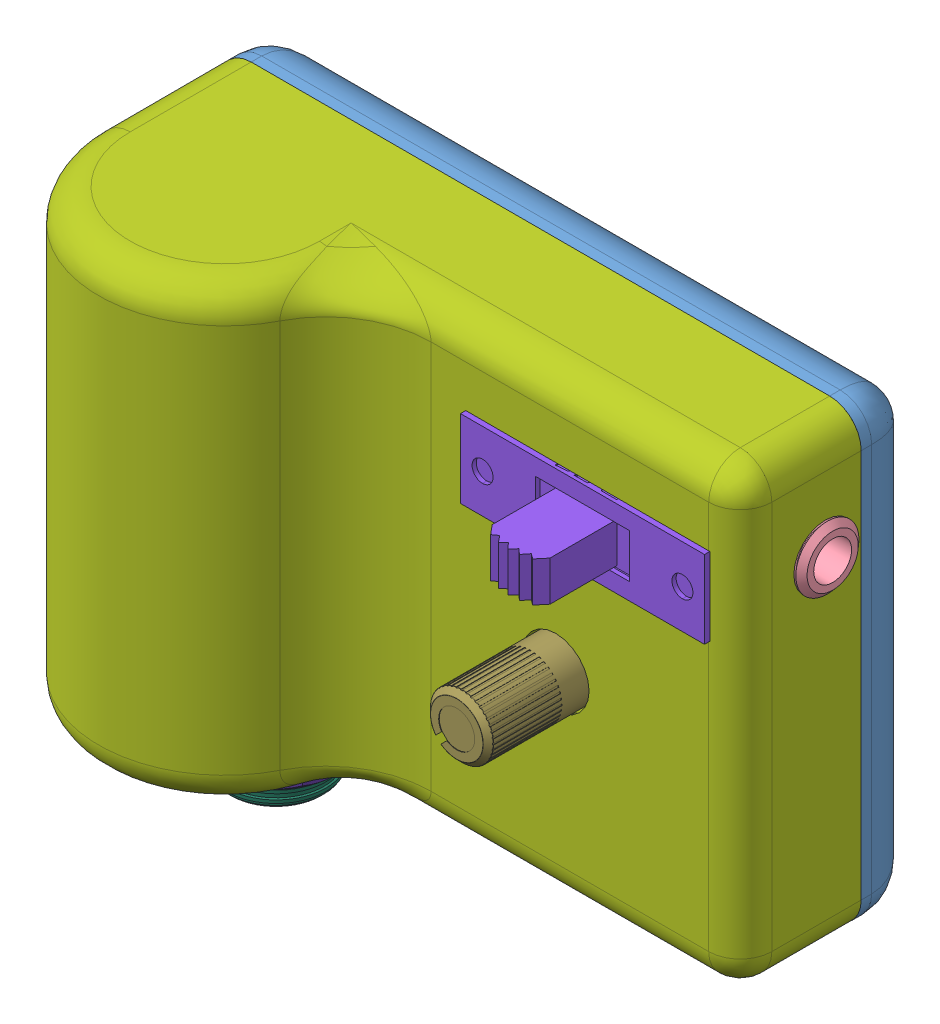
SolidWorks assembly Assem1, configuration Default. Lengths in mm.
Overall size (61.7 49.06 31.9).
226 component instances, 80 part files, 10 mates.
Components (placement in the parent):
- base-1: base [Default] at (33.6508 33.2702 54.2256) size (61 43 11.4)
- Guitar_Headphone_Amp.step-1: Guitar_Headphone_Amp.step [Default] at (133.3435 -10.8718 60.6371) x (0 1 0) z (0 0 1) size (46.1 58.51 24.5)
  - Board.step-1: Board.step [Default] at origin size (37.48 55.26 0.45)
    - Open CASCADE STEP translator 6.8 1.1.1.step-1: Open CASCADE STEP translator 6.8 1.1.1.step [Default] at (0 0 -0.4115) size (37.48 55.26 0.45)
  - U1.step-1: U1.step [Default] at origin size (4 8.8 1.65)
    - 7526814176.step-1: 7526814176.step [Default] at (43.244 100.584 0.1) size (4 8.8 1.65)
      - Extruded.step-1: Extruded.step [Default] at origin size (4 8.8 1.65)
  - R19.step-1: R19.step [Default] at origin size (0.95 1.75 0.55)
    - 7442988304.step-1: 7442988304.step [Default] at (53.086 89.244 0) size (0.95 0.3 0.55)
      - Extruded-0.step-1: Extruded-0.step [Default] at origin size (0.95 0.3 0.55)
    - 7442988304.step-2: 7442988304.step [Default] at (53.086 87.794 0) size (0.95 0.3 0.55)
      - Extruded-0.step-1: Extruded-0.step [Default] at origin size (0.95 0.3 0.55)
    - 7442988144.step-1: 7442988144.step [Default] at (53.086 88.519 0) size (0.95 1.15 0.55)
      - Extruded-1.step-1: Extruded-1.step [Default] at origin size (0.95 1.15 0.55)
  - R18.step-1: R18.step [Default] at origin size (0.95 1.75 0.55)
    - 7442988304.step-1: 7442988304.step [Default] at (57.912 89.244 0) size (0.95 0.3 0.55)
      - Extruded-0.step-1: Extruded-0.step [Default] at origin size (0.95 0.3 0.55)
    - 7442988304.step-2: 7442988304.step [Default] at (57.912 87.794 0) size (0.95 0.3 0.55)
      - Extruded-0.step-1: Extruded-0.step [Default] at origin size (0.95 0.3 0.55)
    - 7442988144.step-1: 7442988144.step [Default] at (57.912 88.519 0) size (0.95 1.15 0.55)
      - Extruded-1.step-1: Extruded-1.step [Default] at origin size (0.95 1.15 0.55)
  - R17.step-1: R17.step [Default] at origin size (1.45 2.2 0.7)
    - 7527189808.step-1: 7527189808.step [Default] at (27.005 91.313 0) size (1.45 1.4 0.7)
      - Extruded-2.step-1: Extruded-2.step [Default] at origin size (1.45 1.4 0.7)
    - 6967077248.step-1: 6967077248.step [Default] at (27.005 90.413 0) size (1.45 0.4 0.7)
      - Extruded-3.step-1: Extruded-3.step [Default] at origin size (1.45 0.4 0.7)
    - 6967077248.step-2: 6967077248.step [Default] at (27.005 92.213 0) size (1.45 0.4 0.7)
      - Extruded-3.step-1: Extruded-3.step [Default] at origin size (1.45 0.4 0.7)
  - R16.step-1: R16.step [Default] at origin size (1.45 2.2 0.6)
    - 7687205168.step-1: 7687205168.step [Default] at (31.7541 82.031 0) size (1.45 0.4 0.6)
      - Extruded-4.step-1: Extruded-4.step [Default] at origin size (1.45 0.4 0.6)
    - 7687205168.step-2: 7687205168.step [Default] at (31.7541 83.831 0) size (1.45 0.4 0.6)
      - Extruded-4.step-1: Extruded-4.step [Default] at origin size (1.45 0.4 0.6)
    - 7687201248.step-1: 7687201248.step [Default] at (31.7541 82.931 0) size (1.45 1.4 0.6)
      - Extruded-5.step-1: Extruded-5.step [Default] at origin size (1.45 1.4 0.6)
  - R15.step-1: R15.step [Default] at origin size (1.45 2.2 0.7)
    - 6967077248.step-1: 6967077248.step [Default] at (27.155 83.301 0) size (1.45 0.4 0.7)
      - Extruded-3.step-1: Extruded-3.step [Default] at origin size (1.45 0.4 0.7)
    - 6967077248.step-2: 6967077248.step [Default] at (27.155 85.101 0) size (1.45 0.4 0.7)
      - Extruded-3.step-1: Extruded-3.step [Default] at origin size (1.45 0.4 0.7)
    - 7527189808.step-1: 7527189808.step [Default] at (27.155 84.201 0) size (1.45 1.4 0.7)
      - Extruded-2.step-1: Extruded-2.step [Default] at origin size (1.45 1.4 0.7)
  - R14.step-1: R14.step [Default] at origin size (1.45 2.2 0.7)
    - 6967077248.step-1: 6967077248.step [Default] at (32.0541 86.095 0) size (1.45 0.4 0.7)
      - Extruded-3.step-1: Extruded-3.step [Default] at origin size (1.45 0.4 0.7)
    - 6967077248.step-2: 6967077248.step [Default] at (32.0541 87.895 0) size (1.45 0.4 0.7)
      - Extruded-3.step-1: Extruded-3.step [Default] at origin size (1.45 0.4 0.7)
    - 7527189808.step-1: 7527189808.step [Default] at (32.0541 86.995 0) size (1.45 1.4 0.7)
      - Extruded-2.step-1: Extruded-2.step [Default] at origin size (1.45 1.4 0.7)
  - R13.step-1: R13.step [Default] at origin size (1.45 2.2 0.7)
    - 6967077248.step-1: 6967077248.step [Default] at (27.155 86.984 0) size (1.45 0.4 0.7)
      - Extruded-3.step-1: Extruded-3.step [Default] at origin size (1.45 0.4 0.7)
    - 6967077248.step-2: 6967077248.step [Default] at (27.155 88.784 0) size (1.45 0.4 0.7)
      - Extruded-3.step-1: Extruded-3.step [Default] at origin size (1.45 0.4 0.7)
    - 7527189808.step-1: 7527189808.step [Default] at (27.155 87.884 0) size (1.45 1.4 0.7)
      - Extruded-2.step-1: Extruded-2.step [Default] at origin size (1.45 1.4 0.7)
  - R12.step-1: R12.step [Default] at origin size (1.45 2.2 0.5)
    - 7553474784.step-1: 7553474784.step [Default] at (32.0541 89.601 0) size (1.45 0.3 0.5)
      - Extruded-6.step-1: Extruded-6.step [Default] at origin size (1.45 0.3 0.5)
    - 7553474784.step-2: 7553474784.step [Default] at (32.0541 91.501 0) size (1.45 0.3 0.5)
      - Extruded-6.step-1: Extruded-6.step [Default] at origin size (1.45 0.3 0.5)
    - 7553476624.step-1: 7553476624.step [Default] at (32.0541 90.551 0) size (1.45 1.6 0.5)
      - Extruded-7.step-1: Extruded-7.step [Default] at origin size (1.45 1.6 0.5)
  - R11.step-1: R11.step [Default] at origin size (1.05 0.55 0.4)
    - 7526808016.step-1: 7526808016.step [Default] at (36.449 80.391 0) x (1 0 0) z (0 0 1) size (1.05 0.55 0.4)
      - Terminal.step-1: Terminal.step [Default] at (-0.525 -0.275 0) size (0.2 0.55 0.4)
        - Open_CASCADE_STEP_translator_6.8_9.2.1.step-1: Open_CASCADE_STEP_translator_6.8_9.2.1.step [Default] at origin size (0.2 0.55 0.4)
      - Terminal.step-2: Terminal.step [Default] at (0.525 0.275 0) x (-1 0 0) z (0 0 1) size (0.2 0.55 0.4)
        - Open_CASCADE_STEP_translator_6.8_9.2.1.step-1: Open_CASCADE_STEP_translator_6.8_9.2.1.step [Default] at origin size (0.2 0.55 0.4)
      - Mid_Body.step-1: Mid_Body.step [Default] at (-0.525 -0.275 0) size (0.97 0.55 0.32)
      - Mark.step-1: Mark.step [Default] at (-0.325 -0.275 0.36) size (0.65 0.55 0.04)
  - R10.step-1: R10.step [Default] at origin size (3.21 1.61 1.81)
    - Res_Stackpole_Electronics_RMCF0805JT220K_eec.step-1: Res_Stackpole_Electronics_RMCF0805JT220K_eec.step [Default] at (39.497 80.01 0) x (1 0 0) z (0 0 1) size (3.21 1.61 1.81)
      - terminals.step-1: terminals.step [Default] at origin size (3.21 1.61 1.81)
      - body.step-1: body.step [Default] at origin size (1.9 1.25 0.55)
      - top.step-1: top.step [Default] at (-0.71 0 0.6) size (1.3 1.25 0.05)
      - logo.step-1: logo.step [Default] at (0 0 0.65) size (0.63 0.29 0.01)
  - R9.step-1: R9.step [Default] at origin size (1.25 2 0.64)
    - Res_Panasonic_ERA6AEB203V_eec.step-1: Res_Panasonic_ERA6AEB203V_eec.step [Default] at (53.213 92.075 0) x (0 1 0) z (0 0 1) size (2 1.25 0.64)
      - terminals-8.step-1: terminals-8.step [Default] at origin size (2 1.25 0.6)
      - alumina_substrate.step-1: alumina_substrate.step [Default] at origin size (1.95 1.25 0.55)
      - coating.step-1: coating.step [Default] at (-0.475 0 0.375) size (1.2 1.04 0.02)
      - logo-9.step-1: logo-9.step [Default] at (0.0109 -0.0405 0.6) size (0.81 0.13 0.07)
  - R8.step-1: R8.step [Default] at origin size (1.25 2 0.5)
    - Res_Vishay_CRCW0805100KFKEA_eec.step-1: Res_Vishay_CRCW0805100KFKEA_eec.step [Default] at (57.618 97.409 0) x (0 1 0) z (0 0 1) size (2 1.25 0.5)
      - body-10.step-1: body-10.step [Default] at (0 0 0.45) x (1 0 0) z (0 0 -1) size (1.9 1.25 0.4)
      - pad.step-1: pad.step [Default] at (-0.8133 -0.625 0.5) x (1 0 0) z (0 1 0) size (0.3 0.5 1.25)
      - pad.step-2: pad.step [Default] at (0.8133 0.625 0.5) x (-1 0 0) z (0 -1 0) size (0.3 0.5 1.25)
      - top-11.step-1: top-11.step [Default] at (0 0 0.05) x (1 0 0) z (0 0 -1) size (1.4 1.25 0.05)
      - top-11.step-2: top-11.step [Default] at (0 0 0.5) x (1 0 0) z (0 0 -1) size (1.4 1.25 0.05)
      - Vishay.step-1: Vishay.step [Default] at (0.032 -0.7832 0.5) size (0.44 0.37 0)
  - R7.step-1: R7.step [Default] at origin size (1.25 2 0.5)
    - Res_Vishay_CRCW0805100KFKEA_eec.step-1: Res_Vishay_CRCW0805100KFKEA_eec.step [Default] at (57.618 101.219 0) x (0 1 0) z (0 0 1) size (2 1.25 0.5)
      - body-10.step-1: body-10.step [Default] at (0 0 0.45) x (1 0 0) z (0 0 -1) size (1.9 1.25 0.4)
      - pad.step-1: pad.step [Default] at (-0.8133 -0.625 0.5) x (1 0 0) z (0 1 0) size (0.3 0.5 1.25)
      - pad.step-2: pad.step [Default] at (0.8133 0.625 0.5) x (-1 0 0) z (0 -1 0) size (0.3 0.5 1.25)
      - top-11.step-1: top-11.step [Default] at (0 0 0.05) x (1 0 0) z (0 0 -1) size (1.4 1.25 0.05)
      - top-11.step-2: top-11.step [Default] at (0 0 0.5) x (1 0 0) z (0 0 -1) size (1.4 1.25 0.05)
      - Vishay.step-1: Vishay.step [Default] at (0.032 -0.7832 0.5) size (0.44 0.37 0)
  - R6.step-1: R6.step [Default] at origin size (11.27 12.64 24.3)
    - Res_Bourns_Inc_PTV09A-4020U-B103_eec.step-1: Res_Bourns_Inc_PTV09A-4020U-B103_eec.step [Default] at (41.402 86.741 0) x (-1 0 0) z (0 0 1) size (11.27 12.64 24.3)
      - body-12.step-1: body-12.step [Default] at origin size (9.42 11.82 8)
      - shell.step-1: shell.step [Default] at origin size (11.27 11 11.4)
      - pins.step-1: pins.step [Default] at origin size (6.5 3.25 6.8)
      - shaft.step-1: shaft.step [Default] at origin size (6 6 14.57)
      - logo-13.step-1: logo-13.step [Default] at (-5 0 6.8) x (0 -1 0) z (-1 0 0) size (8.73 2.81 2.33)
  - R5.step-1: R5.step [Default] at origin size (1.25 2 0.64)
    - Res_Panasonic_ERA6AEB203V_eec.step-1: Res_Panasonic_ERA6AEB203V_eec.step [Default] at (53.213 104.902 0) x (0 1 0) z (0 0 1) size (2 1.25 0.64)
      - terminals-8.step-1: terminals-8.step [Default] at origin size (2 1.25 0.6)
      - alumina_substrate.step-1: alumina_substrate.step [Default] at origin size (1.95 1.25 0.55)
      - coating.step-1: coating.step [Default] at (-0.475 0 0.375) size (1.2 1.04 0.02)
      - logo-9.step-1: logo-9.step [Default] at (0.0109 -0.0405 0.6) size (0.81 0.13 0.07)
  - R4.step-1: R4.step [Default] at origin size (1.25 2 0.64)
    - Res_Panasonic_ERA6AEB203V_eec.step-1: Res_Panasonic_ERA6AEB203V_eec.step [Default] at (57.868 109.855 0) x (0 1 0) z (0 0 1) size (2 1.25 0.64)
      - terminals-8.step-1: terminals-8.step [Default] at origin size (2 1.25 0.6)
      - alumina_substrate.step-1: alumina_substrate.step [Default] at origin size (1.95 1.25 0.55)
      - coating.step-1: coating.step [Default] at (-0.475 0 0.375) size (1.2 1.04 0.02)
      - logo-9.step-1: logo-9.step [Default] at (0.0109 -0.0405 0.6) size (0.81 0.13 0.07)
  - R3.step-1: R3.step [Default] at origin size (1.25 2 0.64)
    - Res_Panasonic_ERA6AEB203V_eec.step-1: Res_Panasonic_ERA6AEB203V_eec.step [Default] at (57.868 114.3 0) x (0 1 0) z (0 0 1) size (2 1.25 0.64)
      - terminals-8.step-1: terminals-8.step [Default] at origin size (2 1.25 0.6)
      - alumina_substrate.step-1: alumina_substrate.step [Default] at origin size (1.95 1.25 0.55)
      - coating.step-1: coating.step [Default] at (-0.475 0 0.375) size (1.2 1.04 0.02)
      - logo-9.step-1: logo-9.step [Default] at (0.0109 -0.0405 0.6) size (0.81 0.13 0.07)
  - R2.step-1: R2.step [Default] at origin size (2.2 1.45 0.5)
    - 7530584752.step-1: 7530584752.step [Default] at (32.827 93.853 0) size (0.3 1.45 0.5)
      - Extruded-14.step-1: Extruded-14.step [Default] at origin size (0.3 1.45 0.5)
    - 7530584752.step-2: 7530584752.step [Default] at (30.927 93.853 0) size (0.3 1.45 0.5)
      - Extruded-14.step-1: Extruded-14.step [Default] at origin size (0.3 1.45 0.5)
    - 7530584992.step-1: 7530584992.step [Default] at (31.877 93.853 0) size (1.6 1.45 0.5)
      - Extruded-15.step-1: Extruded-15.step [Default] at origin size (1.6 1.45 0.5)
  - R1.step-1: R1.step [Default] at origin size (2.1 1.35 0.6)
    - 7553105936.step-1: 7553105936.step [Default] at (27.805 93.98 0) x (1 0 0) z (0 0 1) size (2.1 1.35 0.6)
      - Terminal-1.step-1: Terminal-1.step [Default] at (-1.05 -0.675 0) size (0.15 1.35 0.6)
        - Open_CASCADE_STEP_translator_6.8_3.2.1.step-1: Open_CASCADE_STEP_translator_6.8_3.2.1.step [Default] at origin size (0.15 1.35 0.6)
      - Terminal-1.step-2: Terminal-1.step [Default] at (1.05 0.675 0) x (-1 0 0) z (0 0 1) size (0.15 1.35 0.6)
        - Open_CASCADE_STEP_translator_6.8_3.2.1.step-1: Open_CASCADE_STEP_translator_6.8_3.2.1.step [Default] at origin size (0.15 1.35 0.6)
      - Mid_Body-16.step-1: Mid_Body-16.step [Default] at (-1.05 -0.675 0) size (1.98 1.35 0.48)
      - Mark-17.step-1: Mark-17.step [Default] at (-0.9 -0.675 0.54) size (1.8 1.35 0.06)
  - Q2.step-1: Q2.step [Default] at origin size (1.4 3 1)
    - 7530592512.step-1: 7530592512.step [Default] at (58.293 92.329 0.1) size (1.4 3 1)
      - Extruded-18.step-1: Extruded-18.step [Default] at origin size (1.4 3 1)
  - Q1.step-1: Q1.step [Default] at origin size (2.4 2.92 1.2)
    - Trans_ON_Semiconductor_MMBT2369A_eec.step-1: Trans_ON_Semiconductor_MMBT2369A_eec.step [Default] at (58.693 105.156 0.625) x (-1 0 0) z (0 0 1) size (2.4 2.92 1.2)
      - BAT54S_D87Z_3_PIN.step-1: BAT54S_D87Z_3_PIN.step [Default] at origin size (2.4 2.92 1.2)
      - Onsemi_Updated_Logo.step-1: Onsemi_Updated_Logo.step [Default] at (7.752 -28.0245 0.575) x (-0.003533 -0.999994 0) z (0 0 1) size (1.06 0.24 0)
  - J3.step-1: J3.step [Default] at origin size (11.5 17.5 8.88)
    - Conn_Switchcraft_35RAPC3BH3_eec.step-1: Conn_Switchcraft_35RAPC3BH3_eec.step [Default] at (55.3847 77.2473 0) x (0 1 0) z (0 0 1) size (17.5 11.5 8.88)
      - 1.step-1: 1.step [Default] at (-5.25 -0.25 3) x (0 -1 0) z (1 0 0) size (11.5 8.88 17.5)
        - 1-19.step-1: 1-19.step [Default] at origin size (10 8.5 16.65)
        - 2.step-1: 2.step [Default] at origin size (11.4 1.13 13.9)
        - 35RAPC3BH3.step-1: 35RAPC3BH3.step [Default] at origin size (11.5 5 14)
        - 3.step-1: 3.step [Default] at (5.678 -3.127 14.228) x (1 0 0) z (0 -1 0) size (9.22 11.49 0.51)
        - Switchcraft.step-1: Switchcraft.step [Default] at (5.5 -2.1 -0.28) x (0 1 0) z (1 0 0) size (1.37 5.04 0)
  - J2.step-1: J2.step [Default] at origin size (8 7.1 9.4)
    - Conn_JST_BM02B-PASS-1-TFT_LF_SN_eec.step-1: Conn_JST_BM02B-PASS-1-TFT_LF_SN_eec.step [Default] at (56.261 120.904 0) size (8 7.1 9.4)
      - 1-1.step-1: 1-1.step [Default] x (1 0 0) z (0 -1 0) size (8 9.4 7.1)
        - 1-20.step-1: 1-20.step [Default] at origin size (6.6 5.7 3.2)
        - 2-21.step-1: 2-21.step [Default] at origin size (6.61 2.8 1.7)
        - 3-22.step-1: 3-22.step [Default] at origin size (2.5 3.2 0.5)
        - 4.step-1: 4.step [Default] at origin size (2.5 0.6 1.9)
        - 5.step-1: 5.step [Default] at origin size (8 9.4 5.7)
        - JST.step-1: JST.step [Default] at (4.2787 7.162 -4.0696) x (1 0 0) z (0 1 0) size (1.3 0.63 0.04)
  - J1.step-1: J1.step [Default] at origin size (32.85 18.2 20.01)
    - Conn_Neutrik_NMJ4HFD2_eec.step-1: Conn_Neutrik_NMJ4HFD2_eec.step [Default] at (33.324 116.472 0) x (-1 0 0) z (0 0 1) size (32.85 18.2 20.01)
      - 1-2.step-1: 1-2.step [Default] x (-1 0 0) z (0 0 1) size (32.85 18.2 20.01)
        - 1-23.step-1: 1-23.step [Default] at origin size (32.85 18.2 15.89)
        - 3-24.step-1: 3-24.step [Default] at (-10.9788 0 7.945) x (0 -1 0) z (-1 0 0) size (6.22 2.78 2.54)
        - 4-25.step-1: 4-25.step [Default] at origin size (6.53 15.89 16.01)
        - 2-26.step-1: 2-26.step [Default] at (0.2 0 0) size (15.7 17.47 15.37)
        - 7.step-1: 7.step [Default] at (-7.5104 -9.1 -0.6458) x (1 0 0) z (0 -1 0) size (6.45 1.35 0)
  - FB2.step-1: FB2.step [Default] at origin size (2 1.25 1.05)
    - FBead_Murata_BLM21PG600SZ1J_eec.step-1: FBead_Murata_BLM21PG600SZ1J_eec.step [Default] at (31.6791 79.629 0) x (-1 0 0) z (0 0 1) size (2 1.25 1.05)
      - Electrodes.step-1: Electrodes.step [Default] at origin size (2 1.25 1.05)
      - Dielectric.step-1: Dielectric.step [Default] at origin size (1 1.24 1.04)
      - Murata.step-1: Murata.step [Default] at origin size (0.53 0.12 0)
  - FB1.step-1: FB1.step [Default] at origin size (3.21 1.61 1.81)
    - FBead_Murata_BLM31KN121SH1L_eec.step-1: FBead_Murata_BLM31KN121SH1L_eec.step [Default] at (30.226 76.708 0) x (-1 0 0) z (0 0 1) size (3.21 1.61 1.81)
      - terminals.step-1: terminals.step [Default] at origin size (3.21 1.61 1.81)
      - Center.step-1: Center.step [Default] at origin size (1.8 1.59 1.79)
      - Murata-27.step-1: Murata-27.step [Default] at origin size (0.67 0.15 0)
  - D2.step-1: D2.step [Default] at origin size (1.25 2 0.85)
    - Diode_Taiwan_Semiconductor_TS4148_RYG_eec.step-1: Diode_Taiwan_Semiconductor_TS4148_RYG_eec.step [Default] at (52.963 96.393 0) x (0 1 0) z (0 0 1) size (0.22 1.25 0)
    - Diode_Taiwan_Semiconductor_TS4148_RYG_eec-28.step-1: Diode_Taiwan_Semiconductor_TS4148_RYG_eec-28.step [Default] at (52.963 96.393 0) x (0 1 0) z (0 0 1) size (0.38 0.39 0)
    - Diode_Taiwan_Semiconductor_TS4148_RYG_eec-29.step-1: Diode_Taiwan_Semiconductor_TS4148_RYG_eec-29.step [Default] at (52.963 96.393 0) x (0 1 0) z (0 0 1) size (0.45 1.25 0.85)
    - Diode_Taiwan_Semiconductor_TS4148_RYG_eec-30.step-1: Diode_Taiwan_Semiconductor_TS4148_RYG_eec-30.step [Default] at (52.963 96.393 0) x (0 1 0) z (0 0 1) size (0.45 1.25 0.85)
    - Diode_Taiwan_Semiconductor_TS4148_RYG_eec-31.step-1: Diode_Taiwan_Semiconductor_TS4148_RYG_eec-31.step [Default] at (52.963 96.393 0) x (0 1 0) z (0 0 1) size (1.1 1.25 0.04)
    - Diode_Taiwan_Semiconductor_TS4148_RYG_eec-32.step-1: Diode_Taiwan_Semiconductor_TS4148_RYG_eec-32.step [Default] at (52.963 96.393 0) x (0 1 0) z (0 0 1) size (1.92 1.25 0.77)
  - D1.step-1: D1.step [Default] at origin size (1.25 2 0.85)
    - Diode_Taiwan_Semiconductor_TS4148_RYG_eec.step-1: Diode_Taiwan_Semiconductor_TS4148_RYG_eec.step [Default] at (52.963 101.092 0) x (0 1 0) z (0 0 1) size (0.22 1.25 0)
    - Diode_Taiwan_Semiconductor_TS4148_RYG_eec-28.step-1: Diode_Taiwan_Semiconductor_TS4148_RYG_eec-28.step [Default] at (52.963 101.092 0) x (0 1 0) z (0 0 1) size (0.38 0.39 0)
    - Diode_Taiwan_Semiconductor_TS4148_RYG_eec-29.step-1: Diode_Taiwan_Semiconductor_TS4148_RYG_eec-29.step [Default] at (52.963 101.092 0) x (0 1 0) z (0 0 1) size (0.45 1.25 0.85)
    - Diode_Taiwan_Semiconductor_TS4148_RYG_eec-30.step-1: Diode_Taiwan_Semiconductor_TS4148_RYG_eec-30.step [Default] at (52.963 101.092 0) x (0 1 0) z (0 0 1) size (0.45 1.25 0.85)
    - Diode_Taiwan_Semiconductor_TS4148_RYG_eec-31.step-1: Diode_Taiwan_Semiconductor_TS4148_RYG_eec-31.step [Default] at (52.963 101.092 0) x (0 1 0) z (0 0 1) size (1.1 1.25 0.04)
    - Diode_Taiwan_Semiconductor_TS4148_RYG_eec-32.step-1: Diode_Taiwan_Semiconductor_TS4148_RYG_eec-32.step [Default] at (52.963 101.092 0) x (0 1 0) z (0 0 1) size (1.92 1.25 0.77)
  - C5.step-1: C5.step [Default] at origin size (1.25 2 1.4)
    - Cap_Kemet_C0805C106K8PACTU_eec.step-1: Cap_Kemet_C0805C106K8PACTU_eec.step [Default] at (27.305 80.645 0) x (0 1 0) z (0 0 1) size (0.5 1.25 1.4)
    - Cap_Kemet_C0805C106K8PACTU_eec-33.step-1: Cap_Kemet_C0805C106K8PACTU_eec-33.step [Default] at (27.305 80.645 0) x (0 1 0) z (0 0 1) size (0.5 1.25 1.4)
    - Cap_Kemet_C0805C106K8PACTU_eec-34.step-1: Cap_Kemet_C0805C106K8PACTU_eec-34.step [Default] at (27.305 80.645 0) x (0 1 0) z (0 0 1) size (1 1.15 1.3)
  - C4.step-1: C4.step [Default] at origin size (1.7 0.9 0.9)
    - 6229294720.step-1: 6229294720.step [Default] at (43.18 80.137 0) size (1 0.9 0.9)
      - Extruded-35.step-1: Extruded-35.step [Default] at origin size (1 0.9 0.9)
    - 6229294560.step-1: 6229294560.step [Default] at (43.855 80.137 0) size (0.35 0.9 0.9)
      - Extruded-36.step-1: Extruded-36.step [Default] at origin size (0.35 0.9 0.9)
    - 6229294560.step-2: 6229294560.step [Default] at (42.505 80.137 0) size (0.35 0.9 0.9)
      - Extruded-36.step-1: Extruded-36.step [Default] at origin size (0.35 0.9 0.9)
  - C3.step-1: C3.step [Default] at origin size (1.25 2 1.35)
    - Cap_Murata_GRM21BR61C106KE15K_eec.step-1: Cap_Murata_GRM21BR61C106KE15K_eec.step [Default] at (53.213 109.728 0) x (0 1 0) z (0 0 1) size (2 1.25 1.35)
      - 1-37.step-1: 1-37.step [Default] at origin size (2 1.25 1.35)
      - 2-38.step-1: 2-38.step [Default] at (0 0 0.01) size (1.98 1.23 1.33)
      - Murata_Logo_3.step-1: Murata_Logo_3.step [Default] at (-0.1814 -0.5957 1.2401) size (0.53 0.12 0.1)
  - C2.step-1: C2.step [Default] at origin size (1.25 2 1.35)
    - Cap_Murata_GRM21BR61C106KE15K_eec.step-1: Cap_Murata_GRM21BR61C106KE15K_eec.step [Default] at (53.213 114.3 0) x (0 1 0) z (0 0 1) size (2 1.25 1.35)
      - 1-37.step-1: 1-37.step [Default] at origin size (2 1.25 1.35)
      - 2-38.step-1: 2-38.step [Default] at (0 0 0.01) size (1.98 1.23 1.33)
      - Murata_Logo_3.step-1: Murata_Logo_3.step [Default] at (-0.1814 -0.5957 1.2401) size (0.53 0.12 0.1)
  - C1.step-1: C1.step [Default] at origin size (9.7 8.3 10.5)
    - Cap_Panasonic_EEEFT1E471AP_eec.step-1: Cap_Panasonic_EEEFT1E471AP_eec.step [Default] at (32.252 100.965 0) x (1 0 0) z (0 0 1) size (9.7 8.3 10.5)
      - __X2__FFFDFFFD__X0__8_SIZE_CODE_F.step-1: __X2__FFFDFFFD__X0__8_SIZE_CODE_F.step [Default] x (1 0 0) z (0 -1 0) size (9.7 10.5 8.3)
        - Part2.step-1: Part2.step [Default] at (0 0.6 0) size (8 9.9 8)
        - Part4.step-1: Part4.step [Default] at origin size (8.3 1.6 8.3)
        - Part6.step-1: Part6.step [Default] at (-1.75 0.3 0) size (3.6 1 1)
        - Part6.step-2: Part6.step [Default] at (1.75 0.3 0) x (-1 0 0) z (0 0 -1) size (3.6 1 1)
        - Panasonic.step-1: Panasonic.step [Default] at (2.1831 10.4977 0.0062) x (0 0 -1) z (0 1 0) size (3.29 0.52 0)
- top-2: top [Default] at (27.1508 33.2702 71.7256) x (1 0 0) z (0 0 -1) size (61 43.47 23.5)
- xb-ss-12f26-1: xb-ss-12f26 [Default] at (44.1508 47.2702 48.9256) x (0 -1 0) z (-1 0 0) size (7.44 18.67 23.2)
Mates (geometry in assembly coordinates):
- Coincident1: coincident anti-aligned: plane of base-1 through (6.1508 14.7702 60.2256) normal (0 0 1); plane of Guitar_Headphone_Amp.step-1/Board.step-1/Open CASCADE STEP translator 6.8 1.1.1.step-1 through (7.4865 14.6552 60.2256) normal (0 0 -1)
- Parallel1: parallel anti-aligned: plane of base-1 through (59.0508 52.1202 63.2256) normal (0 -1 0); plane of Guitar_Headphone_Amp.step-1/Board.step-1/Open CASCADE STEP translator 6.8 1.1.1.step-1 through (7.3595 52.1202 60.2256) normal (0 1 0)
- Coincident2: coincident anti-aligned: plane of base-1 through (8.7508 52.1202 63.2256) normal (0 -1 0); plane of Guitar_Headphone_Amp.step-1/Board.step-1/Open CASCADE STEP translator 6.8 1.1.1.step-1 through (7.3595 52.1202 60.2256) normal (0 1 0)
- Lock1: lock: 
- Coincident9: coincident anti-aligned: plane of base-1 through (6.1508 14.7702 60.2256) normal (0 0 1); plane of top-2 through (61.1508 51.7702 60.2256) normal (0 0 -1)
- Coincident10: coincident aligned: plane of base-1 through (64.1508 51.7702 60.2256) normal (1 0 0); plane of top-2 through (64.1508 14.7702 60.2256) normal (1 0 0)
- Coincident11: coincident aligned: plane of base-1 through (6.1508 54.7702 60.2256) normal (0 1 0); plane of top-2 through (61.1508 54.7702 60.2256) normal (0 1 0)
- Coincident12: coincident: plane of top-2 through (61.1508 51.7702 71.7256) normal (0 0 1); plane of xb-ss-12f26-1 through (56.7288 71.0441 71.7256) normal (0 0 -1)
- Coincident14: coincident: plane of top-2 through (57.1508 40.3702 61.7256) normal (-1 0 0); plane of xb-ss-12f26-1 through (57.1508 62.2301 65.7736) normal (1 0 0)
- Coincident15: coincident anti-aligned: plane of top-2 through (57.1508 47.7702 61.7256) normal (0 -1 0); plane of xb-ss-12f26-1 through (56.3628 70.2921 65.923) normal (0 1 0)
